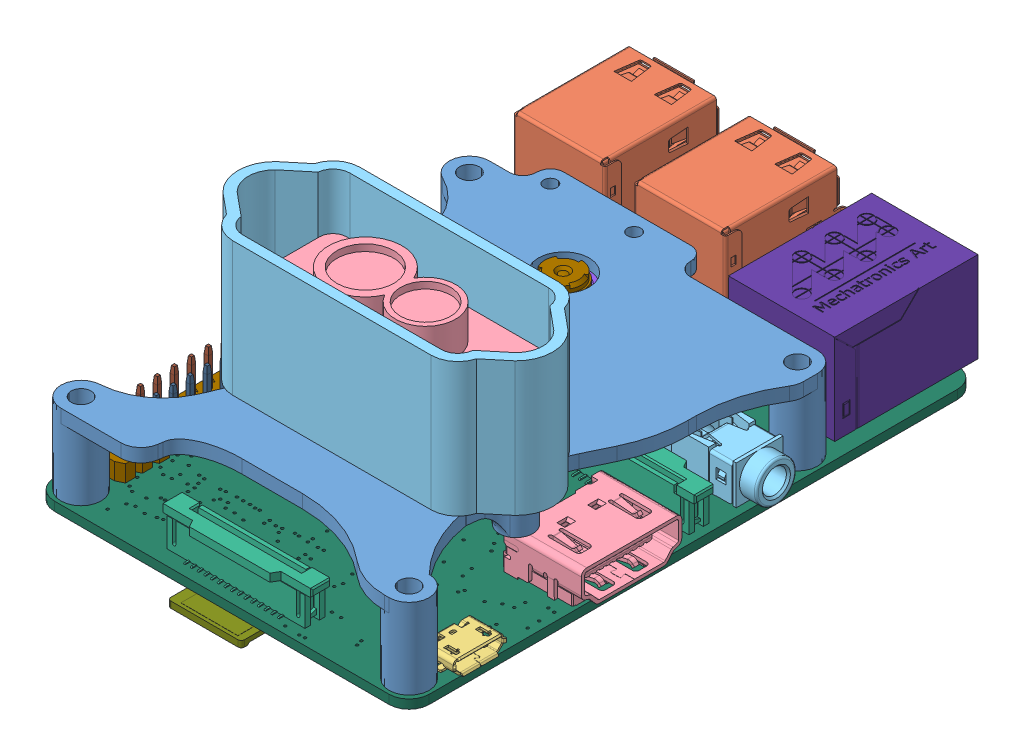
SolidWorks assembly Raspberry pi 3 + kaamera ja lidari kinnitus, configuration Default. Lengths in mm.
Overall size (83 39.33 98.76).
105 component instances, 42 part files, 15 mates.
Components (placement in the parent):
- Kaamera Lidari kinnitus-1: Kaamera Lidari kinnitus [Default] at origin size (55 12.02 68.1)
- Raspberry pi 3 cad model-1: Raspberry pi 3 cad model [Default] at (-40.773 -11 -6.0275) x (0 0 -1) z (0 1 0) size (89.64 57.31 18.59)
  - raspberrypi_3_stripped.step-1: raspberrypi_3_stripped.step [Default] at origin size (89.64 57.31 18.59)
    - RPi3_ModelB v1.step-1: RPi3_ModelB v1.step [Default] at (-6 -61 0) x (1 0 0) z (0 -1 0) size (86.09 18.24 56.14)
      - MOLEX_672983090.step-1: MOLEX_672983090.step [Default] at (30.19 0.8 -64.5) x (0 0 -1) z (1 0 0) size (15.47 17.24 17.92)
      - MOLEX_672983090.step-2: MOLEX_672983090.step [Default] at (30.19 0.8 -82.5) x (0 0 -1) z (1 0 0) size (15.47 17.24 17.92)
      - molex_0473460001.step-1: molex_0473460001.step [Default] at (-31.9 0.8 -37.765) size (7.98 2.76 5.43)
      - molex_0471510001.step-1: molex_0471510001.step [Default] at (-10.5 0.65 -34.125) size (15.04 7.63 12.15)
      - PJ-322.step-1: PJ-322.step [Default] at (11.1 0.8 -42.85) size (7.23 7.55 15)
      - te_1-1734248-5.step-1: te_1-1734248-5.step [Default] at (-38.7109 0.8 -63.5) x (0 0 1) z (-1 0 0) size (22.4 5.68 5.07)
      - te_1-1734248-5.step-2: te_1-1734248-5.step [Default] at (2.058 0.82 -46.9107) x (0 0 -1) z (1 0 0) size (22.4 5.68 5.07)
      - MOLEX_1040310811.step-1: MOLEX_1040310811.step [Default] at (-35.065 -0.3 -63.58) x (0 0 -1) z (-1 0 0) size (11.95 1.45 11.4)
      - raspberry_pi_3(RJ45).step-1: raspberry_pi_3(RJ45).step [Default] at (44.6723 16.4551 -37.9773) x (0 0 -1) z (1 0 0) size (9.5 2.68 12.61)
    - Raspberry Pi 3157.step-1: Raspberry Pi 3157.step [Default] at origin size (50.8 5 2.5)
    - Raspberry Pi 3242.step-1: Raspberry Pi 3242.step [Default] at (0.3 0 0) size (0.64 0.64 5.5)
    - Raspberry Pi 3266.step-1: Raspberry Pi 3266.step [Default] at (0.3 -0.1777 0) size (0.64 0.64 5.5)
    - raspberry_pi_3(bar_180_2x20).step-1: raspberry_pi_3(bar_180_2x20).step [Default] at (-40.3908 28.1775 3.5) x (0 1 0) z (-1 0 0) size (3.19 3.1 48.91)
    - Raspberry Pi 312.step-1: Raspberry Pi 312.step [Default] at origin size (13.97 14.11 1)
    - Raspberry Pi 3180.step-1: Raspberry Pi 3180.step [Default] at origin size (0.5 0.3 0.3)
    - Raspberry Pi 31.step-1: Raspberry Pi 31.step [Default] at origin size (84.92 56 1.33)
    - raspberry_pi_B+_(microsd2).step-1: raspberry_pi_B+_(microsd2).step [Default] at (-43.2065 2.73 -0.97) x (1 0 0) z (0 1 0) size (15 0.97 11)
    - Raspberry Pi 3242.step-2: Raspberry Pi 3242.step [Default] at (2.84 0 0) size (0.64 0.64 5.5)
    - Raspberry Pi 3242.step-3: Raspberry Pi 3242.step [Default] at (5.38 0 0) size (0.64 0.64 5.5)
    - Raspberry Pi 3242.step-4: Raspberry Pi 3242.step [Default] at (7.92 0 0) size (0.64 0.64 5.5)
    - Raspberry Pi 3242.step-5: Raspberry Pi 3242.step [Default] at (10.46 0 0) size (0.64 0.64 5.5)
    - Raspberry Pi 3242.step-6: Raspberry Pi 3242.step [Default] at (13 0 0) size (0.64 0.64 5.5)
    - Raspberry Pi 3242.step-7: Raspberry Pi 3242.step [Default] at (15.54 0 0) size (0.64 0.64 5.5)
    - Raspberry Pi 3242.step-8: Raspberry Pi 3242.step [Default] at (18.08 0 0) size (0.64 0.64 5.5)
    - Raspberry Pi 3242.step-9: Raspberry Pi 3242.step [Default] at (20.62 0 0) size (0.64 0.64 5.5)
    - Raspberry Pi 3242.step-10: Raspberry Pi 3242.step [Default] at (23.16 0 0) size (0.64 0.64 5.5)
    - Raspberry Pi 3242.step-11: Raspberry Pi 3242.step [Default] at (25.7 0 0) size (0.64 0.64 5.5)
    - Raspberry Pi 3242.step-12: Raspberry Pi 3242.step [Default] at (28.24 0 0) size (0.64 0.64 5.5)
    - Raspberry Pi 3242.step-13: Raspberry Pi 3242.step [Default] at (30.78 0 0) size (0.64 0.64 5.5)
    - Raspberry Pi 3242.step-14: Raspberry Pi 3242.step [Default] at (33.32 0 0) size (0.64 0.64 5.5)
    - Raspberry Pi 3242.step-15: Raspberry Pi 3242.step [Default] at (35.86 0 0) size (0.64 0.64 5.5)
    - Raspberry Pi 3242.step-16: Raspberry Pi 3242.step [Default] at (38.4 0 0) size (0.64 0.64 5.5)
    - Raspberry Pi 3242.step-17: Raspberry Pi 3242.step [Default] at (40.94 0 0) size (0.64 0.64 5.5)
    - Raspberry Pi 3242.step-18: Raspberry Pi 3242.step [Default] at (43.48 0 0) size (0.64 0.64 5.5)
    - Raspberry Pi 3242.step-19: Raspberry Pi 3242.step [Default] at (46.02 0 0) size (0.64 0.64 5.5)
    - Raspberry Pi 3242.step-20: Raspberry Pi 3242.step [Default] at (48.56 0 0) size (0.64 0.64 5.5)
    - Raspberry Pi 3266.step-2: Raspberry Pi 3266.step [Default] at (2.84 -0.1777 0) size (0.64 0.64 5.5)
    - Raspberry Pi 3266.step-3: Raspberry Pi 3266.step [Default] at (5.38 -0.1777 0) size (0.64 0.64 5.5)
    - Raspberry Pi 3266.step-4: Raspberry Pi 3266.step [Default] at (7.92 -0.1777 0) size (0.64 0.64 5.5)
    - Raspberry Pi 3266.step-5: Raspberry Pi 3266.step [Default] at (10.46 -0.1777 0) size (0.64 0.64 5.5)
    - Raspberry Pi 3266.step-6: Raspberry Pi 3266.step [Default] at (13 -0.1777 0) size (0.64 0.64 5.5)
    - Raspberry Pi 3266.step-7: Raspberry Pi 3266.step [Default] at (15.54 -0.1777 0) size (0.64 0.64 5.5)
    - Raspberry Pi 3266.step-8: Raspberry Pi 3266.step [Default] at (18.08 -0.1777 0) size (0.64 0.64 5.5)
    - Raspberry Pi 3266.step-9: Raspberry Pi 3266.step [Default] at (20.62 -0.1777 0) size (0.64 0.64 5.5)
    - Raspberry Pi 3266.step-10: Raspberry Pi 3266.step [Default] at (23.16 -0.1777 0) size (0.64 0.64 5.5)
    - Raspberry Pi 3266.step-11: Raspberry Pi 3266.step [Default] at (25.7 -0.1777 0) size (0.64 0.64 5.5)
    - Raspberry Pi 3266.step-12: Raspberry Pi 3266.step [Default] at (28.24 -0.1777 0) size (0.64 0.64 5.5)
    - Raspberry Pi 3266.step-13: Raspberry Pi 3266.step [Default] at (30.78 -0.1777 0) size (0.64 0.64 5.5)
    - Raspberry Pi 3266.step-14: Raspberry Pi 3266.step [Default] at (33.32 -0.1777 0) size (0.64 0.64 5.5)
    - Raspberry Pi 3266.step-15: Raspberry Pi 3266.step [Default] at (35.86 -0.1777 0) size (0.64 0.64 5.5)
    - Raspberry Pi 3266.step-16: Raspberry Pi 3266.step [Default] at (38.4 -0.1777 0) size (0.64 0.64 5.5)
    - Raspberry Pi 3266.step-17: Raspberry Pi 3266.step [Default] at (40.94 -0.1777 0) size (0.64 0.64 5.5)
    - Raspberry Pi 3266.step-18: Raspberry Pi 3266.step [Default] at (43.48 -0.1777 0) size (0.64 0.64 5.5)
    - Raspberry Pi 3266.step-19: Raspberry Pi 3266.step [Default] at (46.02 -0.1777 0) size (0.64 0.64 5.5)
    - Raspberry Pi 3266.step-20: Raspberry Pi 3266.step [Default] at (48.56 -0.1777 0) size (0.64 0.64 5.5)
    - raspberry_pi_B_(RJ45).step-1: raspberry_pi_B_(RJ45).step [Default] at (38.93 -23.19 14.5) x (0 1 0) z (1 0 0) size (15.88 16.5 21.4)
- Raspberry pi CAMERA V2-1: Raspberry pi CAMERA V2 [Default] at (-50.1884 -4.59 -13.2798) x (-1 0 0) z (0 1 0) size (23.86 25 9.96)
  - RspCameraMia.stp-1: RspCameraMia.stp [Default] at origin size (23.86 25 9.96)
    - 70521906.stp-1: 70521906.stp [Default] at (1.7167 0.8597 0.0159) size (2 2.1 0.95)
      - 70521906_01.stp-1: 70521906_01.stp [Default] at origin size (0.25 0.55 0.75)
      - 70521906_02.stp-1: 70521906_02.stp [Default] at origin size (0.25 0.55 0.75)
      - 70521906_03.stp-1: 70521906_03.stp [Default] at origin size (2 1.25 0.9)
      - 70521906_04.stp-1: 70521906_04.stp [Default] at origin size (0.25 0.55 0.75)
      - 70521906_05.stp-1: 70521906_05.stp [Default] at origin size (0.25 0.55 0.75)
      - 70521906_06.stp-1: 70521906_06.stp [Default] at origin size (0.25 0.55 0.75)
      - 70521906_07.stp-1: 70521906_07.stp [Default] at origin size (0.25 0.55 0.75)
    - PicameraPCB.stp-1: PicameraPCB.stp [Default] at (0.2393 -0.0199 0) x (-1 0 0) z (0 0 1) size (23.86 25 2.2)
    - OVA5647_Housing.stp-1: OVA5647_Housing.stp [Default] at (-2.4078 0.0859 1) x (1 0 0) z (0 -1 0) size (8 3.95 8)
    - OVA5647_Lens_FOV.stp-1: OVA5647_Lens_FOV.stp [Default] at (-2.4087 0.0921 5.963) x (1 0 0) z (0 -1 0) size (6 3.35 6)
    - ribbon_cam.stp-1: ribbon_cam.stp [Default] at (-2.4804 0.3633 1.4162) x (0 1 0) z (1 0 0) size (5.6 0.69 4.76)
    - CCD.stp-1: CCD.stp [Default] at (-2.0757 0.287 1.296) x (1 0 0) z (0 -1 0) size (8.01 0.69 8.01)
    - CAPC-0805-T0.75-BN.stp-1: CAPC-0805-T0.75-BN.stp [Default] at (4.562 5.9833 -0.0026) x (0 -1 0) z (0 0 -1) size (2.1 1.35 0.75)
    - CAPC-0805-T0.75-BN.stp-2: CAPC-0805-T0.75-BN.stp [Default] at (2.0233 10.2705 -0.0026) x (0 -1 0) z (0 0 -1) size (2.1 1.35 0.75)
    - CAPC-0402-T0.55-BN.stp-1: CAPC-0402-T0.55-BN.stp [Default] at (-2.9562 6.224 -0.2572) x (-1 0 0) z (0 -1 0) size (1.05 0.55 0.55)
    - CAPC-0402-T0.55-BN.stp-2: CAPC-0402-T0.55-BN.stp [Default] at (-2.9504 5.2898 -0.2691) x (-1 0 0) z (0 -1 0) size (1.05 0.55 0.55)
    - CAPC-0402-T0.55-BN.stp-3: CAPC-0402-T0.55-BN.stp [Default] at (4.5768 -5.1833 -0.2811) x (-1 0 0) z (0 -1 0) size (1.05 0.55 0.55)
    - CAPC-0402-T0.55-BN.stp-4: CAPC-0402-T0.55-BN.stp [Default] at (2.5547 -5.1368 -0.2811) x (-1 0 0) z (0 -1 0) size (1.05 0.55 0.55)
    - CAPC-0402-T0.55-BN.stp-5: CAPC-0402-T0.55-BN.stp [Default] at (2.6129 -9.93 -0.293) x (-1 0 0) z (0 -1 0) size (1.05 0.55 0.55)
    - CAPC-0402-T0.55-BN.stp-6: CAPC-0402-T0.55-BN.stp [Default] at (4.7286 -9.9294 -0.293) x (-1 0 0) z (0 -1 0) size (1.05 0.55 0.55)
    - CAPC-0402-T0.55-BN.stp-7: CAPC-0402-T0.55-BN.stp [Default] at (8.4068 -3.8793 -0.2811) x (-1 0 0) z (0 -1 0) size (1.05 0.55 0.55)
    - CAPC-0402-T0.55-BN.stp-8: CAPC-0402-T0.55-BN.stp [Default] at (9.0088 0.0217 -0.2796) x (0 1 0) z (-1 0 0) size (1.05 0.55 0.55)
    - CAPC-0402-T0.55-BN.stp-9: CAPC-0402-T0.55-BN.stp [Default] at (10.4284 2.6731 -0.3022) x (0 1 0) z (-1 0 0) size (1.05 0.55 0.55)
    - CAPC-0402-T0.55-BN.stp-10: CAPC-0402-T0.55-BN.stp [Default] at (8.2321 1.3259 -0.2838) x (1 0 0) z (0 1 0) size (1.05 0.55 0.55)
    - RESC-0402.stp-1: RESC-0402.stp [Default] at (3.7919 0.0148 -0.0114) x (1 0 0) z (0 0 -1) size (1.05 0.55 0.4)
    - RESC-0402.stp-2: RESC-0402.stp [Default] at (4.1232 2.6296 -0.0028) x (0 -1 0) z (0 0 -1) size (1.05 0.55 0.4)
    - RESC-0402.stp-3: RESC-0402.stp [Default] at (10.5883 -6.2795 -0.0019) x (0 1 0) z (0 0 -1) size (1.05 0.55 0.4)
    - RESC-0603.stp-1: RESC-0603.stp [Default] at (-2.6191 7.0617 -0.0121) x (1 0 0) z (0 0 -1) size (1.7 0.9 0.55)
    - RESC-0603.stp-2: RESC-0603.stp [Default] at (-3.4466 3.0018 -0.0048) x (0 -1 0) z (0 0 -1) size (1.7 0.9 0.55)
    - RESC-1210.stp-1: RESC-1210.stp [Default] at (2.2265 5.9002 -0.0068) x (0 -1 0) z (0 0 -1) size (3.3 2.7 0.6)
    - c-1-1734248-5-e-raspberry_display.stp-1: c-1-1734248-5-e-raspberry_display.stp [Default] at (-10.6651 0.0449 -1.5) x (0 -1 0) z (-1 0 0) size (22.4 3.22 5.68)
    - SOT23-5.stp-1: SOT23-5.stp [Default] at (4.2989 9.8879 0.5457) x (0 -1 0) z (0 0 -1) size (2.84 3.01 1.19)
    - SOT23-5.stp-2: SOT23-5.stp [Default] at (3.5194 -3.2493 0.04) x (-1 0 0) z (0 0 -1) size (2.84 3.01 1.19)
    - SOT23-5.stp-3: SOT23-5.stp [Default] at (3.5816 -8.055 0.0206) x (-1 0 0) z (0 0 -1) size (2.84 3.01 1.19)
    - KX7 SMD Quartz Crystal Resonator 3.2x2.5mm.stp-1: KX7 SMD Quartz Crystal Resonator 3.2x2.5mm.stp [Default] at (9.9746 -4.9221 0.0339) x (-1 0 0) z (0 -1 0) size (3.2 0.6 2.5)
    - c6aaa.stp-1: c6aaa.stp [Default] at (0.0643 0.0942 0) x (1 0 0) z (0 0 -1) size (2 2.99 0.6)
    - 4pin_smd.stp-1: 4pin_smd.stp [Default] at (0.027 0.0676 0) x (1 0 0) z (0 0 -1) size (1.29 1 0.47)
    - 4pin_smd.stp-2: 4pin_smd.stp [Default] at (-0.0093 -6.0092 -0.0198) x (1 0 0) z (0 0 -1) size (1.29 1 0.47)
    - 4pin_smd.stp-3: 4pin_smd.stp [Default] at (0.0326 -3.0068 -0.0235) x (1 0 0) z (0 0 -1) size (1.29 1 0.47)
- TFmini lidar sensor CAD-1: TFmini lidar sensor CAD [Default] at (-41.7231 3 17.9145) x (0 0 -1) z (1 0 0) size (15 16 43)
- Kaamera, aku ja lidari kinnitus-1: Kaamera, aku ja lidari kinnitus [Default] at (-72.6837 -17.33 43.9145) size (83 17 98)
- Lidari kaitse-1: Lidari kaitse [Default] at (-15.4643 2 58.7634) size (47 20 19)
Mates (geometry in assembly coordinates):
- Concentric1: concentric anti-aligned: cylinder of Kaamera Lidari kinnitus-1 through (-67.6837 2 38.9145) axis (0 -1 0) radius 1.48; cylinder of Raspberry pi 3 cad model-1/raspberrypi_3_stripped.step-1/Raspberry Pi 31.step-1 through (-67.6837 -11.75 38.9145) axis (0 1 0) radius 1.375
- Concentric2: concentric anti-aligned: cylinder of Kaamera Lidari kinnitus-1 through (-18.6837 2 -19.0855) axis (0 -1 0) radius 1.48; cylinder of Raspberry pi 3 cad model-1/raspberrypi_3_stripped.step-1/Raspberry Pi 31.step-1 through (-18.6837 -11.75 -19.0855) axis (0 1 0) radius 1.375
- Coincident1: coincident anti-aligned: plane of Kaamera Lidari kinnitus-1 through (-67.6837 -10 38.9145) normal (0 -1 0); plane of Raspberry pi 3 cad model-1/raspberrypi_3_stripped.step-1/Raspberry Pi 31.step-1 through (-15.1737 -10 42.4245) normal (0 1 0)
- Concentric8: concentric aligned: cylinder of TFmini lidar sensor CAD-1 through (-59.7231 3 17.9145) axis (0 -1 0) radius 1.175; circle of Kaamera Lidari kinnitus-1
- Parallel1: parallel anti-aligned: plane of TFmini lidar sensor CAD-1 through (-26.8981 3 10.4145) normal (0 0 -1); plane of Kaamera Lidari kinnitus-1 through (0 2 34.9145) normal (0 0 1)
- Concentric9: concentric: cylinder of Kaamera Lidari kinnitus-1 through (-18.6837 2 38.9145) axis (0 -1 0) radius 1.48; circle of Raspberry kinnitus v1.1-1
- Concentric10: concentric: cylinder of Kaamera Lidari kinnitus-1 through (-67.6837 2 -19.0855) axis (0 -1 0) radius 1.48; cylinder of Raspberry kinnitus v1.1-1 through (-67.6837 -15.33 -19.0855) axis (0 -1 0) radius 1.25
- Coincident4: coincident: plane of Raspberry pi 3 cad model-1/raspberrypi_3_stripped.step-1/Raspberry Pi 31.step-1 through (-71.1837 -11.33 -42.5097) normal (0 -1 0); plane of Raspberry kinnitus v1.1-1 through (-18.6837 -11.33 38.9145) normal (0 1 0)
- Concentric11: concentric aligned: circle of Kaamera Lidari kinnitus-1; circle of Raspberry pi CAMERA V2-1/RspCameraMia.stp-1/PicameraPCB.stp-1
- Concentric12: concentric aligned: circle of Kaamera Lidari kinnitus-1; circle of Raspberry pi CAMERA V2-1/RspCameraMia.stp-1/PicameraPCB.stp-1
- Coincident5: coincident anti-aligned: plane of Kaamera Lidari kinnitus-1 through (0 -3.65 0) normal (0 -1 0); plane of Raspberry pi CAMERA V2-1/RspCameraMia.stp-1/PicameraPCB.stp-1 through (-60.1502 -3.65 -2.7175) normal (0 1 0)
- Concentric13: concentric anti-aligned: cylinder of TFmini lidar sensor CAD-1 through (-23.7231 3 17.9145) axis (0 -1 0) radius 1.175; circle of Lidari kaitse-1
- Coincident6: coincident anti-aligned: plane of Kaamera Lidari kinnitus-1 through (0 2 0) normal (0 1 0); plane of Lidari kaitse-1 through (-56.5481 2 12.4145) normal (0 -1 0)
- Concentric14: concentric aligned: circle of Kaamera Lidari kinnitus-1; circle of Lidari kaitse-1
- Coincident7: coincident anti-aligned: plane of TFmini lidar sensor CAD-1 through (-23.4699 3 17.9145) normal (0 -1 0); plane of Lidari kaitse-1 through (-56.5481 3 12.4145) normal (0 1 0)
